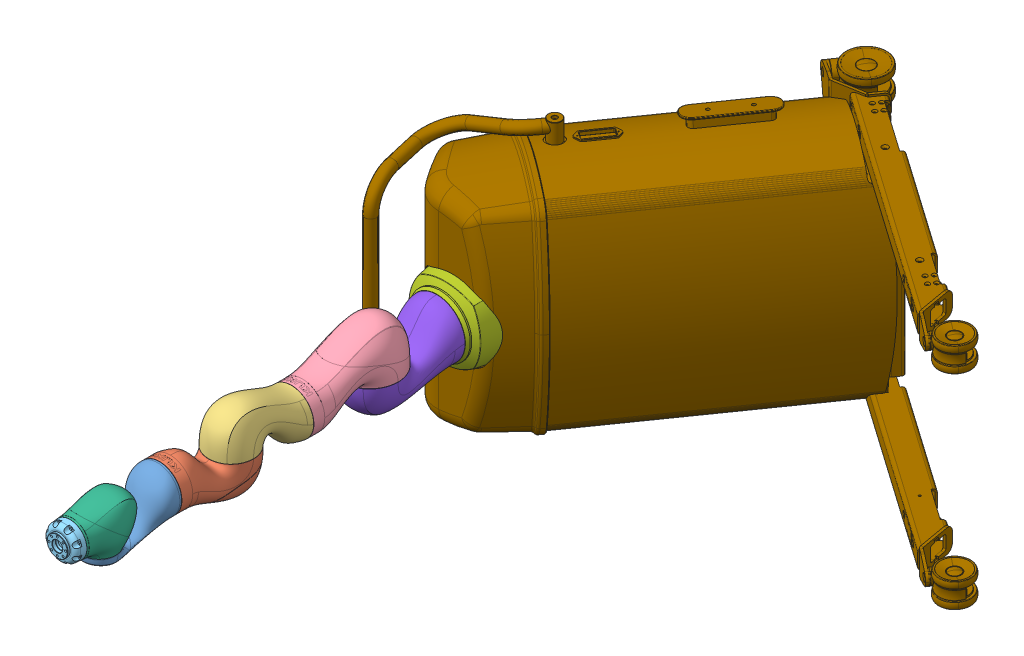
SolidWorks assembly lbrMed_withBase, configuration Default. Lengths in mm.
Overall size (1621.06 766 2244.17).
9 component instances, 9 part files, 3 mates.
Components (placement in the parent):
- Wrist1_body-2: Wrist1_body [Default] at origin size (137.43 170.81 261.47)
- UpperArm_body-1: UpperArm_body [Default] at origin size (137.03 183.96 286.04)
- Elbow_body-1: Elbow_body [Default] at origin size (136.09 183.95 261.22)
- LowerArm_body-1: LowerArm_body [Default] at origin size (171.08 201.65 323.93)
- Wrist3_body-1: Wrist3_body [Default] at origin size (102.25 102.25 38.4)
- Wrist2_body-1: Wrist2_body [Default] at origin size (136.25 137.94 182.79)
- Base_body-1: Base_body [Default] at origin size (277.84 277.84 157.78)
- Shoulder_body-1: Shoulder_body [Default] at origin size (171.08 202.96 299.34)
- only_platform-1: only_platform [Default] at (515.1468 0 -732.7058) x (-0.819152 0 -0.573576) z (0 1 0) size (1151.95 1181.08 766)
Mates (geometry in assembly coordinates):
- Concentric1: concentric: cylinder of Base_body-1 through (84.8528 84.8528 0) axis (0 0 1) radius 5; cylinder of only_platform-1 through (84.8528 84.8528 -125.779) axis (0 0 1) radius 5.25
- Concentric2: concentric: cylinder of Base_body-1 through (84.8528 -84.8528 0) axis (0 0 1) radius 5; cylinder of only_platform-1 through (84.8528 -84.8528 -125.779) axis (0 0 1) radius 5.25
- Coincident1: coincident anti-aligned: plane of Base_body-1 through (0 0 3) normal (0 0 -1); plane of only_platform-1 through (127.5 127.5 3) normal (0 0 1)
